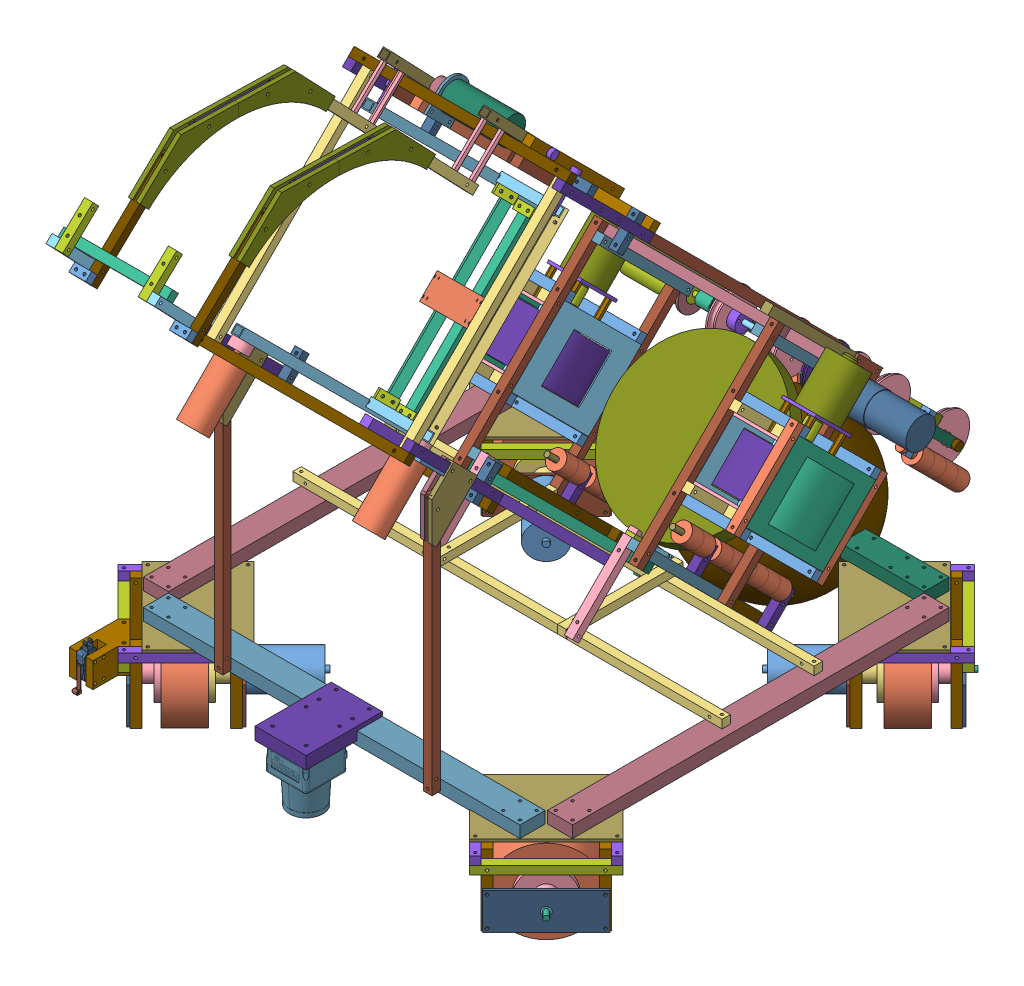
SolidWorks assembly R2, configuration ﾃﾞﾌｫﾙﾄ. Lengths in mm. (continued)
Components (placement in the parent): (continued)
- Copy of Copy of Copy of Copy of Copy of 角材１^R2-1: Copy of Copy of Copy of Copy of Copy of 角材１^R2 [ﾃﾞﾌｫﾙﾄ] at (96.3839 8.5994 989.898) x (0 1 0) z (0 0 -1) size (310 10 10) (virtual)
- Part3^R2-1: Part3^R2 [ﾃﾞﾌｫﾙﾄ] at (103.3839 18.5994 989.898) x (0 1 0) z (1 0 0) size (77.65 54.37 5) (virtual)
- Copy of Part3^R2-4: Copy of Part3^R2 [ﾃﾞﾌｫﾙﾄ] at (94.3981 18.5994 989.898) x (0 1 0) z (1 0 0) size (77.65 54.37 5) (virtual)
- Part3^R2-8: Part3^R2 [ﾃﾞﾌｫﾙﾄ] at (-146.6161 18.5994 989.898) x (0 1 0) z (1 0 0) size (77.65 54.37 5) (virtual)
- Copy of Copy of Copy of Copy of Copy of 角材１^R2-2: Copy of Copy of Copy of Copy of Copy of 角材１^R2 [ﾃﾞﾌｫﾙﾄ] at (-153.6161 8.5994 989.898) x (0 1 0) z (0 0 -1) size (310 10 10) (virtual)
- Copy of Part3^R2-5: Copy of Part3^R2 [ﾃﾞﾌｫﾙﾄ] at (-155.6161 18.5994 989.898) x (0 1 0) z (1 0 0) size (77.65 54.37 5) (virtual)
- Copy of Copy of Part25^R2-1: Copy of Copy of Part25^R2 [ﾃﾞﾌｫﾙﾄ] at (-253.8319 -117.3906 383.8174) x (-1 0 0) z (0 -0.848615 0.529011) size (12 56 56) (hidden, virtual)
- URG-04LX_LN^R2-2: URG-04LX_LN^R2 [ﾃﾞﾌｫﾙﾄ] at (512.2679 -3.342 526.7072) x (0 0 -1) z (1 0 0) size (52.32 70.11 73.77) (hidden, virtual)
- Part4^R2-1: Part4^R2 [ﾃﾞﾌｫﾙﾄ] at (512.2679 -3.442 526.7072) x (0 0 1) z (0 -1 0) size (81.7 49.41 3.02) (hidden, virtual)
- UST-30LX^R2-2: UST-30LX^R2 [ﾃﾞﾌｫﾙﾄ] at (-169.7841 2.0994 439.43) x (0.707107 0 0.707107) z (0.707107 0 -0.707107) size (50.21 70.01 72.52) (virtual)
  - SWP-02205^UST-30LX_R2-1: SWP-02205^UST-30LX_R2 [ﾃﾞﾌｫﾙﾄ] at origin size (50.21 70.01 72.52) (virtual)
  - M2__5.5_TM3022__O______O____^UST-30LX_R2-1: M2__5.5_TM3022__O______O____^UST-30LX_R2 [ﾃﾞﾌｫﾙﾄ] at (16.7 32.3 -24.6969) x (-0.213413 -0.976962 0) z (0 0 -1) size (3.5 3.5 6.1) (virtual)
  - M2__5.5_TM3022__O______O____^UST-30LX_R2-2: M2__5.5_TM3022__O______O____^UST-30LX_R2 [ﾃﾞﾌｫﾙﾄ] at (-16.7 32.3 -24.6969) x (-0.213413 -0.976962 0) z (0 0 -1) size (3.5 3.5 6.1) (virtual)
  - M2__5.5_TM3022__O______O____^UST-30LX_R2-3: M2__5.5_TM3022__O______O____^UST-30LX_R2 [ﾃﾞﾌｫﾙﾄ] at (-16.7 13.9 -24.6969) x (-0.213413 -0.976962 0) z (0 0 -1) size (3.5 3.5 6.1) (virtual)
  - M2__5.5_TM3022__O______O____^UST-30LX_R2-4: M2__5.5_TM3022__O______O____^UST-30LX_R2 [ﾃﾞﾌｫﾙﾄ] at (16.7 13.9 -24.6969) x (-0.213413 -0.976962 0) z (0 0 -1) size (3.5 3.5 6.1) (virtual)
- Part5^R2-1: Part5^R2 [ﾃﾞﾌｫﾙﾄ] at (-169.7841 -7.9006 439.43) x (-0.707107 0 -0.707107) z (0 1 0) size (94 73 30) (virtual)
- Copy of Part5^R2-1: Copy of Part5^R2 [ﾃﾞﾌｫﾙﾄ] at (-23.6161 14.0994 1010.398) x (1 0 0) z (0 1 0) size (61 91 15) (virtual)
- UST-30LX^R2-4: UST-30LX^R2 [ﾃﾞﾌｫﾙﾄ] at (-23.6161 24.0994 1010.398) x (-1 0 0) z (0 0 1) size (50.21 70.01 72.52) (virtual)
  - SWP-02205^UST-30LX_R2-1: SWP-02205^UST-30LX_R2 [ﾃﾞﾌｫﾙﾄ] at origin size (50.21 70.01 72.52) (virtual)
  - M2__5.5_TM3022__O______O____^UST-30LX_R2-1: M2__5.5_TM3022__O______O____^UST-30LX_R2 [ﾃﾞﾌｫﾙﾄ] at (16.7 32.3 -24.6969) x (-0.213413 -0.976962 0) z (0 0 -1) size (3.5 3.5 6.1) (virtual)
  - M2__5.5_TM3022__O______O____^UST-30LX_R2-2: M2__5.5_TM3022__O______O____^UST-30LX_R2 [ﾃﾞﾌｫﾙﾄ] at (-16.7 32.3 -24.6969) x (-0.213413 -0.976962 0) z (0 0 -1) size (3.5 3.5 6.1) (virtual)
  - M2__5.5_TM3022__O______O____^UST-30LX_R2-3: M2__5.5_TM3022__O______O____^UST-30LX_R2 [ﾃﾞﾌｫﾙﾄ] at (-16.7 13.9 -24.6969) x (-0.213413 -0.976962 0) z (0 0 -1) size (3.5 3.5 6.1) (virtual)
  - M2__5.5_TM3022__O______O____^UST-30LX_R2-4: M2__5.5_TM3022__O______O____^UST-30LX_R2 [ﾃﾞﾌｫﾙﾄ] at (16.7 13.9 -24.6969) x (-0.213413 -0.976962 0) z (0 0 -1) size (3.5 3.5 6.1) (virtual)
- Part6^R2-1: Part6^R2 [ﾃﾞﾌｫﾙﾄ] at (-23.6019 -13.4006 449.6189) x (0.102963 -0.774711 0.623876) z (-0.153263 -0.632076 -0.759599) size (190 190 190) (virtual)
- Part7^R2-2: Part7^R2 [ﾃﾞﾌｫﾙﾄ] at (-152.7669 -1289.3445 274.9479) x (-0.707107 0 -0.707107) z (0 1 0) size (80 61 10) (virtual)
- Copy of Copy of Part9^R2-1: Copy of Copy of Part9^R2 [ﾃﾞﾌｫﾙﾄ] at (-21.185 395.6899 817.7908) x (0.7107 0.497446 0.497446) z (0.703495 -0.502541 -0.502541) size (265 30 15) (virtual)
- Copy (3) of Copy of Copy of Copy of Copy of 角材１^R2-2: Copy (3) of Copy of Copy of Copy of Copy of 角材１^R2 [ﾃﾞﾌｫﾙﾄ] at (63.5945 341.9116 960.4016) x (0 0.707107 -0.707107) z (0.703495 -0.502541 -0.502541) size (230 10 10) (virtual)
- Copy of Part9^R2-1: Copy of Part9^R2 [ﾃﾞﾌｫﾙﾄ] at (-18.4519 -0.0628 620.5152) x (0 0.778227 0.627983) z (-1 0 0) size (50 10.5 10) (virtual)
- Copy of Part8^R2-1: Copy of Part8^R2 [ﾃﾞﾌｫﾙﾄ] at (-8.4519 -3.1339 620.4395) x (0 0.707107 0.707107) z (-1 0 0) size (42.8 26.9 30.3) (virtual)
- Copy of D3V-016-1C23^R2-1: Copy of D3V-016-1C23^R2 [ﾃﾞﾌｫﾙﾄ] at (-28.4519 -2.0192 621.0669) x (-1 0 0) z (0 -0.707107 -0.707107) size (10.3 26.4 49.2) (virtual)
  - D3V_016_1C23_BASE^Copy of D3V-016-1C23_R2-1: D3V_016_1C23_BASE^Copy of D3V-016-1C23_R2 [ﾃﾞﾌｫﾙﾄ] at origin size (10.3 19.05 37.8) (virtual)
  - D3V_016_1C23_LEVER^Copy of D3V-016-1C23_R2-1: D3V_016_1C23_LEVER^Copy of D3V-016-1C23_R2 [ﾃﾞﾌｫﾙﾄ] at (-4.8 14.7 -11.8) x (0 0 -1) z (1 0 0) size (28.3 7.35 7.1) (virtual)
  - D3V_016_1C23_BUTTON^Copy of D3V-016-1C23_R2-1: D3V_016_1C23_BUTTON^Copy of D3V-016-1C23_R2 [ﾃﾞﾌｫﾙﾄ] at (-4.85 11.6 2) size (4.3 3.1 2.8) (virtual)
- Part8^R2-2: Part8^R2 [ﾃﾞﾌｫﾙﾄ] at (-309.058 -35.9006 911.726) x (-0.707107 0 -0.707107) z (-0.707107 0 0.707107) size (61.21 30 51.21) (virtual)
- Copy of Copy (2) of Copy of D3V-016-1C23^R2-1: Copy of Copy (2) of Copy of D3V-016-1C23^R2 [ﾃﾞﾌｫﾙﾄ] at (-260.137 -20.9006 1035.0442) x (-1 0 0) z (0 1 0) size (10.3 26.4 49.2) (virtual)
  - D3V_016_1C23_BASE^Copy of Copy (2) of Copy of D3V-016-1C23_R2-1: D3V_016_1C23_BASE^Copy of Copy (2) of Copy of D3V-016-1C23_R2 [ﾃﾞﾌｫﾙﾄ] at origin size (10.3 19.05 37.8) (virtual)
  - D3V_016_1C23_LEVER^Copy of Copy (2) of Copy of D3V-016-1C23_R2-1: D3V_016_1C23_LEVER^Copy of Copy (2) of Copy of D3V-016-1C23_R2 [ﾃﾞﾌｫﾙﾄ] at (-4.8 14.7 -11.8) x (0 0 -1) z (1 0 0) size (28.3 7.35 7.1) (virtual)
  - D3V_016_1C23_BUTTON^Copy of Copy (2) of Copy of D3V-016-1C23_R2-1: D3V_016_1C23_BUTTON^Copy of Copy (2) of Copy of D3V-016-1C23_R2 [ﾃﾞﾌｫﾙﾄ] at (-4.85 11.6 2) size (4.3 3.1 2.8) (virtual)
Mates (geometry in assembly coordinates):
- 距離1: distance = 20 mm anti-aligned: plane of Assem3-1/Copy of Copy of Copy of Copy (2) of Copy of Copy (2) of Copy of Copy (2) of 角材１^Assem3-2 through (-103.6019 41.0994 639.898) normal (0 -1 0); plane of Runner-1/Copy of Part9^Runner-1 through (50.3133 21.0994 988.766) normal (0 1 0)
- 同心円5: concentric aligned: cylinder of Copy of Shooter^R2-1/Copy of Copy of Copy of Copy of Copy (2) of Copy of Copy (2) of 角材１^Shooter-2 through (51.3981 176.9142 460.2355) axis (0 0.707107 -0.707107) radius 1.6; cylinder of Rail-1/Copy (2) of Copy of Copy of Copy of Copy of 角材１^Rail-4 through (51.3981 185.3994 451.7502) axis (0 0.707107 -0.707107) radius 1.6
- 同心円6: concentric aligned: cylinder of Copy of Shooter^R2-1/Copy of Copy of Copy of Copy of Copy (2) of Copy of Copy (2) of 角材１^Shooter-2 through (-98.6019 176.9142 460.2355) axis (0 0.707107 -0.707107) radius 1.6; cylinder of Rail-1/Copy (2) of Copy of Copy of Copy of Copy of 角材１^Rail-3 through (-98.6019 185.3994 451.7502) axis (0 0.707107 -0.707107) radius 1.6
- 距離5: distance = 2 mm anti-aligned: plane of Assem1-1/Copy (2) of Copy of Copy of Copy of Copy of 角材１^Assem1-3 through (-93.6019 174.7928 455.2857) normal (0 -0.707107 0.707107); plane of Assem3-1/Copy of Copy of Copy of Copy of Copy (2) of Copy of Copy (2) of 角材１^Assem3-2 through (-133.6019 180.4497 463.771) normal (0 0.707107 -0.707107)
- 距離6: distance = 200 mm aligned: plane of Assem3-1/Copy of Copy of Copy of Copy (2) of Copy of Copy (2) of Copy of Copy (2) of 角材１^Assem3-1 through (46.3981 51.0994 779.898) normal (0 0 1); plane of Runner-1/Copy of Part9^Runner-1 through (-248.6161 6.0994 979.898) normal (0 0 1)
- 同心円12: concentric aligned: cylinder of Copy of Runner^R2-1/Copy of Part9^Runner-1 through (101.3839 13.5994 949.898) axis (0 0 1) radius 1.6; cylinder of Copy of Copy of Copy of Copy of Copy of 角材１^Assem4-1 through (101.3839 13.5994 989.898) axis (0 0 1) radius 1.6
- 平行1: parallel aligned: plane of Copy of Rail^R2-1/Copy of 角材１^Rail-1 through (106.3981 270.9594 910.6625) normal (1 0 0); plane of Copy of Copy of Copy of Copy of Copy of 角材１^Assem4-1 through (106.3839 8.5994 979.898) normal (1 0 0)
- 一致16: coincident anti-aligned: plane of Copy of Runner^R2-1/Copy of Part9^Runner-1 through (-248.6161 6.0994 979.898) normal (0 0 1); plane of Copy of Copy of Copy of Copy of Copy of 角材１^Assem4-1 through (96.3839 8.5994 979.898) normal (0 0 -1)
- 同心円15: concentric aligned: cylinder of Copy of Copy of Copy of Copy of Copy of 角材１^Assem4-1 through (96.3839 303.5994 984.898) axis (-1 0 0) radius 1.6; cylinder of Part3^R2-1 through (108.3839 303.5994 984.898) axis (-1 0 0) radius 1.75
- 一致20: coincident anti-aligned: plane of Copy of Copy of Copy of Copy of Copy of 角材１^Assem4-1 through (106.3839 8.5994 979.898) normal (1 0 0); plane of Part3^R2-1 through (106.3839 18.5994 989.898) normal (-1 0 0)
- 平行2: parallel anti-aligned: plane of Copy of Copy of Copy of Copy of Copy of 角材１^Assem4-1 through (96.3839 8.5994 989.898) normal (0 0 1); plane of Part3^R2-1 through (106.3839 18.5994 989.998) normal (0 0 -1)
- 同心円16: concentric anti-aligned: cylinder of Copy of Rail^R2-1/Copy of 角材１^Rail-1 through (106.3981 313.3858 946.0178) axis (1 0 0) radius 1.6; cylinder of Copy of Part3^R2-4 through (99.3981 313.3858 946.0178) axis (-1 0 0) radius 1.75
- 同心円17: concentric anti-aligned: cylinder of Copy of Rail^R2-1/Copy of 角材１^Rail-1 through (106.3981 334.599 967.231) axis (1 0 0) radius 1.6; cylinder of Copy of Part3^R2-4 through (99.3981 334.599 967.231) axis (-1 0 0) radius 1.75
- 一致21: coincident anti-aligned: plane of Copy of Rail^R2-1/Copy of 角材１^Rail-1 through (96.3981 270.9594 910.6625) normal (-1 0 0); plane of Copy of Part3^R2-4 through (96.3981 18.5994 989.898) normal (1 0 0)
- 平行3: parallel aligned: cylinder of Part3^R2-1 through (108.3839 303.5994 984.898) axis (-1 0 0) radius 1.75; cylinder of Copy of Part3^R2-4 through (99.3981 303.5994 984.898) axis (-1 0 0) radius 1.75
- 一致22: coincident anti-aligned: plane of Part3^R2-8 through (-143.6161 18.5994 989.898) normal (-1 0 0); plane of Copy of Copy of Copy of Copy of Copy of 角材１^R2-2 through (-143.6161 8.5994 979.898) normal (1 0 0)
- 同心円19: concentric aligned: cylinder of Part3^R2-8 through (-141.6161 303.5994 984.898) axis (-1 0 0) radius 1.75; cylinder of Copy of Copy of Copy of Copy of Copy of 角材１^R2-2 through (-153.6161 303.5994 984.898) axis (-1 0 0) radius 1.6
- 平行4: parallel anti-aligned: plane of Part3^R2-8 through (-143.6161 18.5994 989.998) normal (0 0 -1); plane of Copy of Copy of Copy of Copy of Copy of 角材１^R2-2 through (-153.6161 8.5994 989.898) normal (0 0 1)
- 平行5: parallel aligned: cylinder of Part3^R2-8 through (-141.6161 303.5994 984.898) axis (-1 0 0) radius 1.75; cylinder of Copy of Part3^R2-5 through (-150.6161 303.5994 984.898) axis (-1 0 0) radius 1.75
- 同心円20: concentric aligned: cylinder of Copy of Runner^R2-1/Copy of Part9^Runner-1 through (-148.6161 13.5994 949.898) axis (0 0 1) radius 1.6; cylinder of Copy of Copy of Copy of Copy of Copy of 角材１^R2-2 through (-148.6161 13.5994 989.898) axis (0 0 1) radius 1.6
- 同心円21: concentric aligned: cylinder of Part3^R2-8 through (-141.6161 303.5994 984.898) axis (-1 0 0) radius 1.75; cylinder of Copy of Part3^R2-5 through (-150.6161 303.5994 984.898) axis (-1 0 0) radius 1.75
- 同心円22: concentric aligned: cylinder of Part3^R2-8 through (-141.6161 334.599 967.231) axis (-1 0 0) radius 1.75; cylinder of Copy of Part3^R2-5 through (-150.6161 334.599 967.231) axis (-1 0 0) radius 1.75
- 一致23: coincident anti-aligned: plane of Copy of Copy of Copy of Copy of Copy of 角材１^R2-2 through (-153.6161 8.5994 979.898) normal (-1 0 0); plane of Copy of Part3^R2-5 through (-153.6161 18.5994 989.898) normal (1 0 0)
- 平行9: parallel anti-aligned: plane of Copy of Rail^R2-1/Copy of 角材１^Rail-2 through (-153.6019 270.9594 910.6625) normal (-1 0 0); plane of Copy of Part3^R2-5 through (-153.6161 18.5994 989.898) normal (1 0 0)
- 一致24: coincident anti-aligned: plane of Copy of Runner^R2-1/Copy of Part9^Runner-1 through (-248.6161 6.0994 979.898) normal (0 0 1); plane of Copy of Copy of Copy of Copy of Copy of 角材１^R2-2 through (-153.6161 8.5994 979.898) normal (0 0 -1)
- 相対固定2: in place: plane of ? through (147.9801 484.6223 447.7831) normal (0 -1 0); plane of ? through (0 484.6223 0) normal (0 -1 0); moOrthogonalPlaneRef_w of ? through (147.9801 484.6223 447.7831) normal (0 -1 0); plane of ? through (0 484.6223 0) normal (0 0 -1); plane of ? through (147.9801 484.6223 447.7831) normal (0 -1 0); plane of ? through (0 484.6223 0) normal (-1 0 0); plane of URG-04LX_LN^R2-2 through (488.5179 -3.442 502.9572) normal (0 -1 0); unknown of Part4^R2-1
- 一致26: coincident aligned: plane of ?; plane of ?
- 一致27: coincident aligned: moOrthogonalPlaneRef_w of URG-04LX_LN^R2-2; plane of Part4^R2-1 through (512.2679 -3.442 526.7072) normal (-1 0 0)
- 一致28: coincident anti-aligned: moOrthogonalPlaneRef_w of URG-04LX_LN^R2-2 through (-3.442 526.7072 0) axis (0 -1 0); plane of Part4^R2-1 through (512.2679 -3.442 526.7072) normal (0 0 1)
- 相対固定3: in place: plane of ? through (-388.8532 -195.8752 405.8314) normal (0 -1 0); plane of ? through (0 -195.8752 0) normal (0 -1 0); plane of ? through (-388.8532 -195.8752 405.8314) normal (0 -1 0); plane of ? through (0 -195.8752 0) normal (0 0 -1); plane of ? through (-388.8532 -195.8752 405.8314) normal (0 -1 0); plane of ? through (0 -195.8752 0) normal (-1 0 0); plane of UST-30LX^R2-2/SWP-02205^UST-30LX_R2-1 through (-169.7841 -7.9006 439.43) normal (0 1 0); unknown of Part5^R2-1
- 一致27: coincident aligned: plane of ?; plane of ?
- 一致28: coincident aligned: moOrthogonalPlaneRef_w of UST-30LX^R2-2/SWP-02205^UST-30LX_R2-1; plane of Part5^R2-1 through (-169.7841 -7.9006 439.43) normal (-0.707107 0 0.707107)
- 一致29: coincident anti-aligned: moOrthogonalPlaneRef_w of UST-30LX^R2-2/SWP-02205^UST-30LX_R2-1; plane of Part5^R2-1 through (-169.7841 -7.9006 439.43) normal (-0.707107 0 -0.707107)
- 相対固定4: in place: plane of ? through (-1289.4289 1471.9298 338.742) normal (0 1 0); plane of ? through (-1289.4289 1471.9298 338.742) normal (0 1 0); plane of ? through (-1289.4289 1471.9298 338.742) normal (0 0 1); unknown of ?; plane of ? through (-1289.4289 1471.9298 338.742) normal (-1 0 0); unknown of ?; plane of Copy of Part5^R2-1 through (-23.6161 14.0994 1010.398) normal (0 1 0); unknown of UST-30LX^R2-4/SWP-02205^UST-30LX_R2-1
- 一致31: coincident aligned: plane of ?; plane of ?
- 一致32: coincident aligned: plane of Copy of Part5^R2-1 through (-23.6161 14.0994 1010.398) normal (0 0 -1); moOrthogonalPlaneRef_w of UST-30LX^R2-4/SWP-02205^UST-30LX_R2-1 through (-23.6161 14.0994 1010.398) axis (0 0 -1)
- 一致33: coincident anti-aligned: plane of Copy of Part5^R2-1 through (-23.6161 14.0994 1010.398) normal (1 0 0); moOrthogonalPlaneRef_w of UST-30LX^R2-4/SWP-02205^UST-30LX_R2-1
- 一致35: coincident aligned: plane of Copy of Runner^R2-1/Copy of Part9^Runner-1 through (-248.6161 6.0994 949.898) normal (0 0 -1); plane of Copy of Part5^R2-1 through (-23.6161 21.0994 949.898) normal (0 0 -1)
- 一致36: coincident aligned: plane of Copy of Runner^R2-1/Part9^Runner-1 through (232.7981 21.0994 498.4838) normal (1 0 0); plane of Shooter-1/Copy of Copy (4) of Copy of Copy of Copy of Copy (2) of Copy of Copy (2) of 角材１^Shooter-1 through (232.7981 31.0994 759.898) normal (1 0 0)
- 正接4: tangent aligned: sphere of Part6^R2-1
- 正接5: tangent: circle of Copy of Shooter^R2-1/Part20^Shooter-12; unknown of Part6^R2-1
- 正接6: tangent: circle of Copy of Shooter^R2-1/Part20^Shooter-3; unknown of Part6^R2-1
- 一致39: coincident anti-aligned: plane of Copy of Runner^R2-1/Copy of Part9^Runner-1 through (50.3133 21.0994 988.766) normal (0 1 0); plane of Copy of Part5^R2-1 through (-23.6161 21.0994 1010.398) normal (0 -1 0)
- 同心円27: concentric anti-aligned: cylinder of Copy of Runner^R2-1/Copy of Copy of 足回り角^Runner-1/Copy of Part6^Copy of Copy of 足回り角_Runner-7 through (-222.8171 -0.9006 432.3589) axis (-0.707107 0 0.707107) radius 1.6; cylinder of Part5^R2-1 through (-221.4029 -0.9006 430.9447) axis (0.707107 0 -0.707107) radius 1.75
- 同心円28: concentric anti-aligned: cylinder of Copy of Runner^R2-1/Copy of Copy of 足回り角^Runner-1/Copy of Part6^Copy of Copy of 足回り角_Runner-7 through (-162.7131 -0.9006 492.463) axis (-0.707107 0 0.707107) radius 1.6; cylinder of Part5^R2-1 through (-161.2989 -0.9006 491.0488) axis (0.707107 0 -0.707107) radius 1.75
- 一致41: coincident anti-aligned: plane of Copy of Runner^R2-1/Copy of Copy of 足回り角^Runner-1/Copy of Copy of Part6^Copy of Copy of 足回り角_Runner-4 through (-160.2798 -87.5752 509.0384) normal (0.707107 0 -0.707107); plane of Part5^R2-1 through (-199.8362 -7.9006 469.482) normal (-0.707107 0 0.707107)
- 同心円29: concentric aligned: cylinder of Copy of Runner^R2-1/Copy of Part9^Runner-1 through (-43.6161 6.0994 954.898) axis (0 1 0) radius 1.6; cylinder of Copy of Part5^R2-1 through (-43.6161 21.0994 954.898) axis (0 1 0) radius 1.75
- 一致43: coincident anti-aligned: plane of Copy of Rail^R2-1/Copy of Copy (2) of Copy of Copy of Copy of Copy of Copy of Copy of Copy of Copy (2) of Copy of Copy (9) of Copy (2) of 角材１^Rail-1 through (95.5761 371.3678 975.7156) normal (0.703495 -0.502541 -0.502541); plane of Copy (3) of Copy of Copy of Copy of Copy of 角材１^R2-2 through (63.5945 341.9116 960.4016) normal (-0.703495 0.502541 0.502541)
- 同心円34: concentric aligned: cylinder of Copy of Rail^R2-1/Copy of Copy of Copy of Copy of 角材１^Rail-1 through (-114.0806 291.7963 761.7939) axis (-0.703495 0.502541 0.502541) radius 1.75; cylinder of Copy of Copy of Part9^R2-1 through (-114.0806 291.7963 761.7939) axis (-0.703495 0.502541 0.502541) radius 1.6
- 同心円36: concentric aligned: cylinder of Copy of Rail^R2-1/Copy of Copy of Copy of Copy of 角材１^Rail-1 through (-114.0806 305.9385 747.6517) axis (-0.703495 0.502541 0.502541) radius 1.75; cylinder of Copy of Copy of Part9^R2-1 through (-114.0806 305.9385 747.6517) axis (-0.703495 0.502541 0.502541) radius 1.6
- 一致44: coincident anti-aligned: plane of Copy of Rail^R2-1/Copy of Copy of Copy of Copy of 角材１^Rail-1 through (-117.6341 215.0629 833.5528) normal (-0.703495 0.502541 0.502541); plane of Copy of Copy of Part9^R2-1 through (-10.6326 388.1517 810.2527) normal (0.703495 -0.502541 -0.502541)
- 一致45: coincident anti-aligned: plane of Copy of Part9^R2-1 through (-18.4519 -0.0628 620.5152) normal (1 0 0); plane of Copy of Part8^R2-1 through (-18.4519 -21.6768 605.3691) normal (-1 0 0)
- 一致46: coincident anti-aligned: plane of Copy of Part8^R2-1 through (-28.7519 -21.6768 605.3691) normal (1 0 0); plane of Copy of D3V-016-1C23^R2-1/D3V_016_1C23_BASE^Copy of D3V-016-1C23_R2-1 through (-28.7519 -2.0192 621.6326) normal (-1 0 0)
- 同心円37: concentric aligned: cylinder of Copy of Part8^R2-1 through (-38.7519 -2.0192 621.0669) axis (-1 0 0) radius 1.75; cylinder of Copy of D3V-016-1C23^R2-1/D3V_016_1C23_BASE^Copy of D3V-016-1C23_R2-1 through (-18.7519 -2.0192 621.0669) axis (-1 0 0) radius 1.7
- 同心円38: concentric aligned: cylinder of Copy of Part8^R2-1 through (-38.7519 -10.4338 598.0859) axis (-1 0 0) radius 1.75; cylinder of Copy of D3V-016-1C23^R2-1/D3V_016_1C23_BASE^Copy of D3V-016-1C23_R2-1 through (-18.7519 -10.4338 598.0859) axis (-1 0 0) radius 1.55
- 同心円39: concentric anti-aligned: cylinder of Copy of Part9^R2-1 through (-28.4519 -0.8878 591.6513) axis (1 0 0) radius 1.75; cylinder of Copy of Part8^R2-1 through (-8.4519 -0.8878 591.6513) axis (-1 0 0) radius 1.75
- 一致47: coincident anti-aligned: plane of Copy of Shooter^R2-1/Copy (3) of Copy of Copy of Copy of Copy of Copy (2) of Copy of Copy (2) of 角材１^Shooter-1 through (-103.6019 -59.9666 548.6238) normal (0 0.707107 -0.707107); plane of Copy of Part8^R2-1 through (-38.7519 10.7441 619.3345) normal (0 -0.707107 0.707107)
- 同心円40: concentric aligned: cylinder of Copy of Shooter^R2-1/Copy (4) of Copy of Copy of Copy of Copy of Copy (2) of Copy of Copy (2) of 角材１^Shooter-2 through (-13.6019 14.2796 622.87) axis (0 0.707107 -0.707107) radius 1.6; cylinder of Copy of Part8^R2-1 through (-13.6019 5.0518 632.0978) axis (0 0.707107 -0.707107) radius 1.75
- 同心円41: concentric aligned: cylinder of Copy of Shooter^R2-1/Copy (4) of Copy of Copy of Copy of Copy of Copy (2) of Copy of Copy (2) of 角材１^Shooter-2 through (-33.6019 14.2796 622.87) axis (0 0.707107 -0.707107) radius 1.6; cylinder of Copy of Part8^R2-1 through (-33.6019 5.0518 632.0978) axis (0 0.707107 -0.707107) radius 1.75
- 一致53: coincident anti-aligned: plane of Copy of Runner^R2-1/Copy of Copy of 足回り角^Runner-3/Part6^Copy of Copy of 足回り角_Runner-12 through (-233.4237 -5.9006 1025.2153) normal (-0.707107 0 0.707107); plane of Part8^R2-2 through (-327.9855 -35.9006 930.6535) normal (0.707107 0 -0.707107)
- 一致54: coincident anti-aligned: plane of Copy of Runner^R2-1/Copy of Copy of 足回り角^Runner-3/Part6^Copy of Copy of 足回り角_Runner-12 through (-336.0361 -5.9006 934.5406) normal (0 1 0); plane of Part8^R2-2 through (-268.7791 -5.9006 989.8599) normal (0 -1 0)
- 一致55: coincident anti-aligned: plane of Copy of Runner^R2-1/Copy of Copy of 足回り角^Runner-3/Copy of Part6^Copy of Copy of 足回り角_Runner-9 through (-240.4948 -5.9006 1018.1442) normal (-0.707107 0 -0.707107); plane of Part8^R2-2 through (-221.5673 4.0994 999.2167) normal (0.707107 0 0.707107)
- 同心円46: concentric aligned: cylinder of Part8^R2-2 through (-218.4237 -20.9006 1035.0442) axis (-1 0 0) radius 1.75; cylinder of Copy of Copy (2) of Copy of D3V-016-1C23^R2-1/D3V_016_1C23_BASE^Copy of Copy (2) of Copy of D3V-016-1C23_R2-1 through (-250.437 -20.9006 1035.0442) axis (-1 0 0) radius 1.7
- 同心円47: concentric aligned: cylinder of Part8^R2-2 through (-218.4237 1.2994 1045.3442) axis (-1 0 0) radius 1.75; cylinder of Copy of Copy (2) of Copy of D3V-016-1C23^R2-1/D3V_016_1C23_BASE^Copy of Copy (2) of Copy of D3V-016-1C23_R2-1 through (-250.437 1.2994 1045.3442) axis (-1 0 0) radius 1.55
- 一致57: coincident anti-aligned: plane of Part8^R2-2 through (-260.137 4.0994 1023.1442) normal (1 0 0); plane of Copy of Copy (2) of Copy of D3V-016-1C23^R2-1/D3V_016_1C23_BASE^Copy of Copy (2) of Copy of D3V-016-1C23_R2-1 through (-260.137 1.2994 1045.3442) normal (-1 0 0)
